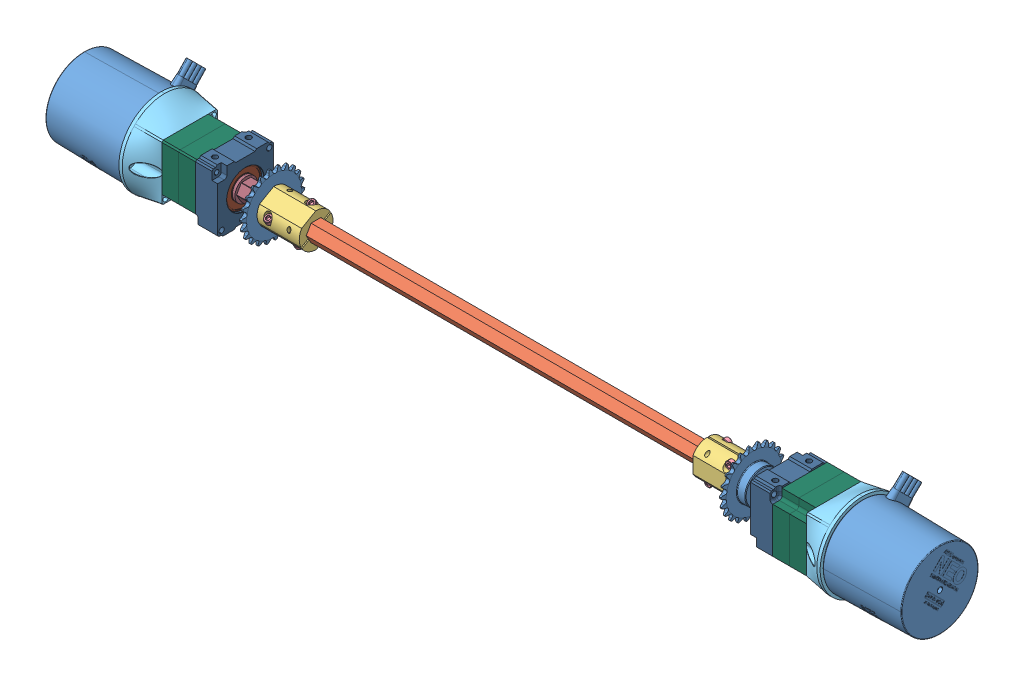
SolidWorks assembly elevator motors, configuration Default. Lengths in mm.
Overall size (645.18 70.15 70.15).
85 component instances, 19 part files, 27 mates.
Components (placement in the parent):
- 22t 25chain gear-1: 22t 25chain gear [Default] at (47.9906 -700.1428 1835.7253) x (-1 0 0) z (0 0.939892 -0.341472) size (9.18 48.36 48.44)
- 22t 25chain gear-2: 22t 25chain gear [Default] at (707.3859 453.67 -162.8689) x (1 0 0) z (0 0.174223 0.984706) size (9.18 48.36 48.44)
- 12in .5hex-1: 12in .5hex [Default] at (534.901 182.7836 1013.2629) x (0 0.972924 0.231127) z (-1 0 0) size (14.05 14.27 317.5)
- TTB-0055 - Half Inch Hex Coupler.stp-1: TTB-0055 - Half Inch Hex Coupler.stp [Default] at (230.101 182.8852 1013.3216) x (0 0.5 -0.866025) z (-1 0 0) size (26 22.23 31.75)
  - 6-32 Hex Coupler.stp-1: 6-32 Hex Coupler.stp [Default] at origin size (25.37 10.53 31.75)
  - 6-32 Hex Coupler.stp-2: 6-32 Hex Coupler.stp [Default] at (0 0 31.75) x (1 0 0) z (0 0 -1) size (25.37 10.53 31.75)
  - 91251A146_Black-Oxide Alloy Steel Socket Head Screw.stp-1: 91251A146_Black-Oxide Alloy Steel Socket Head Screw.stp [Default] at (9.5758 -1.5621 7.9375) x (0.375209 0 0.92694) z (0 -1 0) size (5.74 5.74 13.03)
  - 91251A146_Black-Oxide Alloy Steel Socket Head Screw.stp-2: 91251A146_Black-Oxide Alloy Steel Socket Head Screw.stp [Default] at (9.5758 1.5621 23.8125) x (-0.044233 0 -0.999021) z (0 1 0) size (5.74 5.74 13.03)
  - 91251A146_Black-Oxide Alloy Steel Socket Head Screw.stp-3: 91251A146_Black-Oxide Alloy Steel Socket Head Screw.stp [Default] at (-9.5758 -1.5621 23.8125) x (1 0 0) z (0 -1 0) size (5.74 5.74 13.03)
  - 91251A146_Black-Oxide Alloy Steel Socket Head Screw.stp-4: 91251A146_Black-Oxide Alloy Steel Socket Head Screw.stp [Default] at (-9.5758 1.5621 7.9375) x (1 0 0) z (0 1 0) size (5.74 5.74 13.03)
- TTB-0055 - Half Inch Hex Coupler.stp-2: TTB-0055 - Half Inch Hex Coupler.stp [Default] at (525.2756 182.8852 1013.3216) x (0 1 0) z (1 0 0) size (26 22.23 31.75)
  - 6-32 Hex Coupler.stp-1: 6-32 Hex Coupler.stp [Default] at origin size (25.37 10.53 31.75)
  - 6-32 Hex Coupler.stp-2: 6-32 Hex Coupler.stp [Default] at (0 0 31.75) x (1 0 0) z (0 0 -1) size (25.37 10.53 31.75)
  - 91251A146_Black-Oxide Alloy Steel Socket Head Screw.stp-1: 91251A146_Black-Oxide Alloy Steel Socket Head Screw.stp [Default] at (9.5758 -1.5621 7.9375) x (0.375209 0 0.92694) z (0 -1 0) size (5.74 5.74 13.03)
  - 91251A146_Black-Oxide Alloy Steel Socket Head Screw.stp-2: 91251A146_Black-Oxide Alloy Steel Socket Head Screw.stp [Default] at (9.5758 1.5621 23.8125) x (-0.044233 0 -0.999021) z (0 1 0) size (5.74 5.74 13.03)
  - 91251A146_Black-Oxide Alloy Steel Socket Head Screw.stp-3: 91251A146_Black-Oxide Alloy Steel Socket Head Screw.stp [Default] at (-9.5758 -1.5621 23.8125) x (1 0 0) z (0 -1 0) size (5.74 5.74 13.03)
  - 91251A146_Black-Oxide Alloy Steel Socket Head Screw.stp-4: 91251A146_Black-Oxide Alloy Steel Socket Head Screw.stp [Default] at (-9.5758 1.5621 7.9375) x (1 0 0) z (0 1 0) size (5.74 5.74 13.03)
- VersaPlanetary CIM Adapter (217-4018).step-1: VersaPlanetary CIM Adapter (217-4018).step [Default] at (630.4008 182.9868 1013.2629) x (0 0 1) z (0 -1 0) size (64.01 21.63 64.01)
- VersaPlanetary CIM Adapter (217-4018).step-2: VersaPlanetary CIM Adapter (217-4018).step [Default] at (124.9758 182.9868 1013.2629) x (0 0 1) z (0 1 0) size (64.01 21.63 64.01)
- Copy of Copy (2) of Assem5^elevator motors-1: Copy of Copy (2) of Assem5^elevator motors [Default] at (160.2008 205.2118 1013.2629) x (1 0 0) z (0 0 -1) size (98.55 51.52 52.65) (virtual)
  - 217-2820 Rev1_Public.step-1: 217-2820 Rev1_Public.step [Default] at (-4.6546 22.225 0) x (0 -0.456494 0.889726) z (-1 0 0) size (39.22 38.88 17.4)
    - 217-2625-100.step-1: 217-2625-100.step [Default] at origin size (39.22 38.88 12.7)
      - 217-2625-008 Rev1.step-1: 217-2625-008 Rev1.step [Default] at origin size (34.7 34.7 4.7)
      - 217-2625-010 Rev1.step-1: 217-2625-010 Rev1.step [Default] at (0 10.193 3.65) x (0.999813 0.019336 0) z (0 0 1) size (4 4 12)
      - 217-2625-010 Rev1.step-2: 217-2625-010 Rev1.step [Default] at (8.691 -5.3258 3.65) size (4 4 12)
      - 217-2625-010 Rev1.step-3: 217-2625-010 Rev1.step [Default] at (-8.691 -5.3258 3.65) size (4 4 12)
      - 217-2625-005 Rev1_Planet_Revolving_Follower01.step-1: 217-2625-005 Rev1_Planet_Revolving_Follower01.step [Default] at (8.691 -5.3258 6.35) x (0.932816 0.360354 0) z (0 0 1) size (16.89 16.89 8)
      - 217-2625-005 Rev1_Planet_Revolving_Follower01.step-2: 217-2625-005 Rev1_Planet_Revolving_Follower01.step [Default] at (-8.691 -5.3258 6.35) x (-0.932788 -0.360426 0) z (0 0 1) size (16.89 16.89 8)
      - 217-2625-005 Rev1_Planet_Revolving_Follower01.step-3: 217-2625-005 Rev1_Planet_Revolving_Follower01.step [Default] at (0 10.193 6.35) x (0.893583 0.448898 0) z (0 0 1) size (16.89 16.89 8)
    - 217-2625-007 Rev1_Public.step-1: 217-2625-007 Rev1_Public.step [Default] at (0 0 6.7) x (0.992772 0.120019 0) z (0 0 1) size (15.27 15.27 12.7)
  - 217-2820 Rev1_Public.step-2: 217-2820 Rev1_Public.step [Default] at (-17.15 22.225 0) x (0 0.184082 0.982911) z (-1 0 0) size (39.22 38.88 17.4)
    - 217-2625-100.step-1: 217-2625-100.step [Default] at origin size (39.22 38.88 12.7)
      - 217-2625-008 Rev1.step-1: 217-2625-008 Rev1.step [Default] at origin size (34.7 34.7 4.7)
      - 217-2625-010 Rev1.step-1: 217-2625-010 Rev1.step [Default] at (0 10.193 3.65) x (0.999813 0.019336 0) z (0 0 1) size (4 4 12)
      - 217-2625-010 Rev1.step-2: 217-2625-010 Rev1.step [Default] at (8.691 -5.3258 3.65) size (4 4 12)
      - 217-2625-010 Rev1.step-3: 217-2625-010 Rev1.step [Default] at (-8.691 -5.3258 3.65) size (4 4 12)
      - 217-2625-005 Rev1_Planet_Revolving_Follower01.step-1: 217-2625-005 Rev1_Planet_Revolving_Follower01.step [Default] at (8.691 -5.3258 6.35) x (0.932816 0.360354 0) z (0 0 1) size (16.89 16.89 8)
      - 217-2625-005 Rev1_Planet_Revolving_Follower01.step-2: 217-2625-005 Rev1_Planet_Revolving_Follower01.step [Default] at (-8.691 -5.3258 6.35) x (-0.932788 -0.360426 0) z (0 0 1) size (16.89 16.89 8)
      - 217-2625-005 Rev1_Planet_Revolving_Follower01.step-3: 217-2625-005 Rev1_Planet_Revolving_Follower01.step [Default] at (0 10.193 6.35) x (0.893583 0.448898 0) z (0 0 1) size (16.89 16.89 8)
    - 217-2625-007 Rev1_Public.step-1: 217-2625-007 Rev1_Public.step [Default] at (0 0 6.7) x (0.992772 0.120019 0) z (0 0 1) size (15.27 15.27 12.7)
  - 217-2625-026 Rev1.step-1: 217-2625-026 Rev1.step [Default] at (-6.5 22.225 0) x (0 -1 0) z (-1 0 0) size (44.45 42 18.12)
  - 217-2742-001 Rev4.step-1: 217-2742-001 Rev4.step [Default] at (0.2002 22.225 0) x (1 0 0) z (0 -0.092627 0.995701) size (7 28 28)
  - 217-2742-001 Rev4.step-2: 217-2742-001 Rev4.step [Default] at (8.2002 22.225 0) size (7 28 28)
  - 217-2625-017 Rev1_9714K61.step-1: 217-2625-017 Rev1_9714K61.step [Default] at (7.42 22.3002 -0.342) x (0 0.56703 0.823697) z (0 -0.823697 0.56703) size (28.51 4.98 27.43)
  - 217-2625-003 Rev1.step-1: 217-2625-003 Rev1.step [Default] at (7.4478 22.225 0) x (0 -1 0) z (1 0 0) size (17 17 64.11)
  - 217-2625-018 Rev1_98541A410.step-1: 217-2625-018 Rev1_98541A410.step [Default] at (-0.7046 22.225 0) x (1 0 0) z (0 -0.017452 0.999848) size (1 19.6 17.4)
  - 217-2816-001 Rev1.step-1: 217-2816-001 Rev1.step [Default] at (-6.35 22.225 0) x (0 -1 0) z (1 0 0) size (42 42 14.51)
  - 217-2816-001 Rev1.step-2: 217-2816-001 Rev1.step [Default] at (-19.05 22.225 0) x (0 -1 0) z (1 0 0) size (42 42 14.51)
  - 217-4649-001 Rev1.step-1: 217-4649-001 Rev1.step [Default] at (-32.746 22.225 0) x (0 -1 0) z (1 0 0) size (18 18 13)
  - 217-4649-007 Rev1_94105A824.step-1: 217-4649-007 Rev1_94105A824.step [Default] at (-38.221 22.225 -6.7835) x (-0.996104 -0.088191 0) z (0 0 -1) size (4.83 4.83 4.77)
  - 217-2625-011 Rev1.step-1: 217-2625-011 Rev1.step [Default] at (-37.4818 22.225 0) x (0 0 1) z (0 -1 0) size (8.01 7.5 7.94)
- Copy of Copy of Assem5^elevator motors-1: Copy of Copy of Assem5^elevator motors [Default] at (595.1758 205.2118 1013.2629) x (-1 0 0) z (0 0 1) size (98.55 51.52 52.65) (virtual)
  - 217-2820 Rev1_Public.step-1: 217-2820 Rev1_Public.step [Default] at (-4.6546 22.225 0) x (0 -0.456494 0.889726) z (-1 0 0) size (39.22 38.88 17.4)
    - 217-2625-100.step-1: 217-2625-100.step [Default] at origin size (39.22 38.88 12.7)
      - 217-2625-008 Rev1.step-1: 217-2625-008 Rev1.step [Default] at origin size (34.7 34.7 4.7)
      - 217-2625-010 Rev1.step-1: 217-2625-010 Rev1.step [Default] at (0 10.193 3.65) x (0.999813 0.019336 0) z (0 0 1) size (4 4 12)
      - 217-2625-010 Rev1.step-2: 217-2625-010 Rev1.step [Default] at (8.691 -5.3258 3.65) size (4 4 12)
      - 217-2625-010 Rev1.step-3: 217-2625-010 Rev1.step [Default] at (-8.691 -5.3258 3.65) size (4 4 12)
      - 217-2625-005 Rev1_Planet_Revolving_Follower01.step-1: 217-2625-005 Rev1_Planet_Revolving_Follower01.step [Default] at (8.691 -5.3258 6.35) x (0.932816 0.360354 0) z (0 0 1) size (16.89 16.89 8)
      - 217-2625-005 Rev1_Planet_Revolving_Follower01.step-2: 217-2625-005 Rev1_Planet_Revolving_Follower01.step [Default] at (-8.691 -5.3258 6.35) x (-0.932788 -0.360426 0) z (0 0 1) size (16.89 16.89 8)
      - 217-2625-005 Rev1_Planet_Revolving_Follower01.step-3: 217-2625-005 Rev1_Planet_Revolving_Follower01.step [Default] at (0 10.193 6.35) x (0.893583 0.448898 0) z (0 0 1) size (16.89 16.89 8)
    - 217-2625-007 Rev1_Public.step-1: 217-2625-007 Rev1_Public.step [Default] at (0 0 6.7) x (0.992772 0.120019 0) z (0 0 1) size (15.27 15.27 12.7)
  - 217-2820 Rev1_Public.step-2: 217-2820 Rev1_Public.step [Default] at (-17.15 22.225 0) x (0 0.184082 0.982911) z (-1 0 0) size (39.22 38.88 17.4)
    - 217-2625-100.step-1: 217-2625-100.step [Default] at origin size (39.22 38.88 12.7)
      - 217-2625-008 Rev1.step-1: 217-2625-008 Rev1.step [Default] at origin size (34.7 34.7 4.7)
      - 217-2625-010 Rev1.step-1: 217-2625-010 Rev1.step [Default] at (0 10.193 3.65) x (0.999813 0.019336 0) z (0 0 1) size (4 4 12)
      - 217-2625-010 Rev1.step-2: 217-2625-010 Rev1.step [Default] at (8.691 -5.3258 3.65) size (4 4 12)
      - 217-2625-010 Rev1.step-3: 217-2625-010 Rev1.step [Default] at (-8.691 -5.3258 3.65) size (4 4 12)
      - 217-2625-005 Rev1_Planet_Revolving_Follower01.step-1: 217-2625-005 Rev1_Planet_Revolving_Follower01.step [Default] at (8.691 -5.3258 6.35) x (0.932816 0.360354 0) z (0 0 1) size (16.89 16.89 8)
      - 217-2625-005 Rev1_Planet_Revolving_Follower01.step-2: 217-2625-005 Rev1_Planet_Revolving_Follower01.step [Default] at (-8.691 -5.3258 6.35) x (-0.932788 -0.360426 0) z (0 0 1) size (16.89 16.89 8)
      - 217-2625-005 Rev1_Planet_Revolving_Follower01.step-3: 217-2625-005 Rev1_Planet_Revolving_Follower01.step [Default] at (0 10.193 6.35) x (0.893583 0.448898 0) z (0 0 1) size (16.89 16.89 8)
    - 217-2625-007 Rev1_Public.step-1: 217-2625-007 Rev1_Public.step [Default] at (0 0 6.7) x (0.992772 0.120019 0) z (0 0 1) size (15.27 15.27 12.7)
  - 217-2625-026 Rev1.step-1: 217-2625-026 Rev1.step [Default] at (-6.5 22.225 0) x (0 -1 0) z (-1 0 0) size (44.45 42 18.12)
  - 217-2742-001 Rev4.step-1: 217-2742-001 Rev4.step [Default] at (0.2002 22.225 0) x (1 0 0) z (0 -0.092627 0.995701) size (7 28 28)
  - 217-2742-001 Rev4.step-2: 217-2742-001 Rev4.step [Default] at (8.2002 22.225 0) size (7 28 28)
  - 217-2625-017 Rev1_9714K61.step-1: 217-2625-017 Rev1_9714K61.step [Default] at (7.42 22.3002 -0.342) x (0 0.56703 0.823697) z (0 -0.823697 0.56703) size (28.51 4.98 27.43)
  - 217-2625-003 Rev1.step-1: 217-2625-003 Rev1.step [Default] at (7.4478 22.225 0) x (0 -1 0) z (1 0 0) size (17 17 64.11)
  - 217-2625-018 Rev1_98541A410.step-1: 217-2625-018 Rev1_98541A410.step [Default] at (-0.7046 22.225 0) x (1 0 0) z (0 -0.017452 0.999848) size (1 19.6 17.4)
  - 217-2816-001 Rev1.step-1: 217-2816-001 Rev1.step [Default] at (-6.35 22.225 0) x (0 -1 0) z (1 0 0) size (42 42 14.51)
  - 217-2816-001 Rev1.step-2: 217-2816-001 Rev1.step [Default] at (-19.05 22.225 0) x (0 -1 0) z (1 0 0) size (42 42 14.51)
  - 217-4649-001 Rev1.step-1: 217-4649-001 Rev1.step [Default] at (-32.746 22.225 0) x (0 -1 0) z (1 0 0) size (18 18 13)
  - 217-4649-007 Rev1_94105A824.step-1: 217-4649-007 Rev1_94105A824.step [Default] at (-38.221 22.225 -6.7835) x (-0.996104 -0.088191 0) z (0 0 -1) size (4.83 4.83 4.77)
  - 217-2625-011 Rev1.step-1: 217-2625-011 Rev1.step [Default] at (-37.4818 22.225 0) x (0 0 1) z (0 -1 0) size (8.01 7.5 7.94)
- REV-21-1650-V1.1.step-1: REV-21-1650-V1.1.step [Default] at (113.4508 182.9868 1013.2629) x (0 -1 0) z (1 0 0) size (68.13 68.01 93.35)
- REV-21-1650-V1.1.step-2: REV-21-1650-V1.1.step [Default] at (641.9258 182.9868 1013.2629) x (0 0 1) z (-1 0 0) size (68.13 68.01 93.35)
Mates (geometry in assembly coordinates):
- Coincident149: coincident anti-aligned: plane of Copy of Copy (2) of Assem5^Assem2_short elevator(1)-1/217-2625-003 Rev1.step-1 through (217.401 182.9868 1005.9306) normal (0 0.5 -0.866025); plane of 22t 25chain gear-1 through (189.1742 189.3495 1009.6041) normal (0 -0.5 0.866025)
- Coincident150: coincident anti-aligned: plane of Copy of Copy (2) of Assem5^Assem2_short elevator(1)-1/217-2625-003 Rev1.step-1 through (217.401 176.6368 1009.5967) normal (0 -0.5 -0.866025); plane of 22t 25chain gear-1 through (189.1742 182.9868 1005.9306) normal (0 0.5 0.866025)
- Coincident151: coincident anti-aligned: plane of TTB-0055 - Half Inch Hex Coupler.stp-1/6-32 Hex Coupler.stp-2 through (198.351 182.8852 1013.3216) normal (-1 0 0); plane of 22t 25chain gear-1 through (198.351 182.9868 1013.2776) normal (1 0 0)
- Coincident146: coincident anti-aligned: plane of Copy of Copy of Assem5^Assem2_short elevator(1)-1/217-2625-003 Rev1.step-1 through (537.9756 189.3368 1016.9291) normal (0 1 0); plane of 22t 25chain gear-2 through (566.2023 189.3368 1009.4941) normal (0 -1 0)
- Coincident147: coincident anti-aligned: plane of 12in .5hex-1 through (217.401 182.7836 1005.9306) normal (0 -0.5 -0.866025); plane of 22t 25chain gear-2 through (566.2023 176.6114 1009.4941) normal (0 0.5 0.866025)
- Coincident148: coincident anti-aligned: plane of TTB-0055 - Half Inch Hex Coupler.stp-2/6-32 Hex Coupler.stp-1 through (557.0256 182.8852 1013.3216) normal (1 0 0); plane of 22t 25chain gear-2 through (557.0256 182.9741 1013.1676) normal (-1 0 0)
- Coincident141: coincident anti-aligned: plane of TTB-0055 - Half Inch Hex Coupler.stp-2/6-32 Hex Coupler.stp-1 through (525.2756 182.8852 1005.8719) normal (0 0.5 0.866025); plane of 12in .5hex-1 through (217.401 182.7836 1005.9306) normal (0 -0.5 -0.866025)
- Coincident143: coincident anti-aligned: plane of TTB-0055 - Half Inch Hex Coupler.stp-2/6-32 Hex Coupler.stp-1 through (525.2756 176.4336 1009.5967) normal (0 1 0); plane of 12in .5hex-1 through (217.401 176.4336 1009.5967) normal (0 -1 0)
- Coincident145: coincident anti-aligned: plane of Copy of Copy (2) of Assem5^Assem2_short elevator(1)-1/217-2625-003 Rev1.step-1 through (217.401 176.6368 1009.5967) normal (1 0 0); plane of 12in .5hex-1 through (217.401 182.7836 1013.2629) normal (-1 0 0)
- Coincident137: coincident anti-aligned: plane of Copy of Copy (2) of Assem5^Assem2_short elevator(1)-1/217-2625-003 Rev1.step-1 through (217.401 189.3368 1009.5967) normal (0 1 0); plane of TTB-0055 - Half Inch Hex Coupler.stp-1/6-32 Hex Coupler.stp-1 through (230.101 189.3368 1009.5967) normal (0 -1 0)
- Coincident138: coincident anti-aligned: plane of Copy of Copy (2) of Assem5^Assem2_short elevator(1)-1/217-2625-003 Rev1.step-1 through (217.401 182.9868 1005.9306) normal (0 0.5 -0.866025); plane of TTB-0055 - Half Inch Hex Coupler.stp-1/6-32 Hex Coupler.stp-1 through (230.101 182.8852 1005.8719) normal (0 -0.5 0.866025)
- Distance23: distance = 12.7 mm: plane of Copy of Copy (2) of Assem5^Assem2_short elevator(1)-1/217-2625-003 Rev1.step-1 through (217.401 176.6368 1009.5967) normal (1 0 0); line of TTB-0055 - Half Inch Hex Coupler.stp-1/6-32 Hex Coupler.stp-1 through (230.101 189.3368 1017.0464) axis (0 -0.866025 0.5)
- Coincident135: coincident anti-aligned: plane of Copy of Copy of Assem5^Assem2_short elevator(1)-1/217-2625-003 Rev1.step-1 through (537.9756 189.3368 1009.5967) normal (0 0.5 -0.866025); plane of TTB-0055 - Half Inch Hex Coupler.stp-2/6-32 Hex Coupler.stp-1 through (525.2756 189.3368 1009.5967) normal (0 -0.5 0.866025)
- Coincident136: coincident anti-aligned: plane of Copy of Copy of Assem5^Assem2_short elevator(1)-1/217-2625-003 Rev1.step-1 through (537.9756 189.3368 1016.9291) normal (0 1 0); plane of TTB-0055 - Half Inch Hex Coupler.stp-2/6-32 Hex Coupler.stp-1 through (525.2756 189.3368 1017.0464) normal (0 -1 0)
- Distance24: distance = 12.7 mm aligned: plane of Copy of Copy of Assem5^Assem2_short elevator(1)-1/217-2625-003 Rev1.step-1 through (537.9756 176.6368 1016.9291) normal (-1 0 0); plane of TTB-0055 - Half Inch Hex Coupler.stp-2/6-32 Hex Coupler.stp-2 through (525.2756 182.8852 1013.3216) normal (-1 0 0)
- Concentric11: concentric anti-aligned: circle of Copy of Copy of Assem5^Assem2_short elevator(1)-1/217-2816-001 Rev1.step-2; circle of VersaPlanetary CIM Adapter (217-4018).step-1
- Coincident128: coincident anti-aligned: plane of Copy of Copy of Assem5^Assem2_short elevator(1)-1/217-2816-001 Rev1.step-2 through (620.5758 203.9868 992.2629) normal (1 0 0); plane of VersaPlanetary CIM Adapter (217-4018).step-1 through (620.5758 182.9868 1013.2629) normal (-1 0 0)
- Coincident129: coincident aligned: line of Copy of Copy of Assem5^Assem2_short elevator(1)-1/217-2816-001 Rev1.step-2 through (620.5758 203.9868 1027.2629) axis (0 0 -1); line of VersaPlanetary CIM Adapter (217-4018).step-1 through (620.5758 203.9868 1033.2629) axis (0 0 -1)
- Concentric12: concentric aligned: circle of REV-21-1650-V1.1.step-2; circle of VersaPlanetary CIM Adapter (217-4018).step-1
- Concentric13: concentric aligned: cylinder of REV-21-1650-V1.1.step-2 through (641.9258 182.9868 987.8629) axis (-1 0 0) radius 2.0193; circle of VersaPlanetary CIM Adapter (217-4018).step-1
- Coincident131: coincident anti-aligned: plane of REV-21-1650-V1.1.step-2 through (641.9258 182.9868 1013.2629) normal (-1 0 0); plane of VersaPlanetary CIM Adapter (217-4018).step-1 through (641.9258 182.9868 1013.2629) normal (1 0 0)
- Concentric14: concentric anti-aligned: circle of Copy of Copy (2) of Assem5^Assem2_short elevator(1)-1/217-2816-001 Rev1.step-2; circle of VersaPlanetary CIM Adapter (217-4018).step-2
- Perpendicular3: perpendicular: line of Copy of Copy (2) of Assem5^Assem2_short elevator(1)-1/217-2816-001 Rev1.step-2 through (134.8008 203.9868 999.2629) axis (0 0 1); line of VersaPlanetary CIM Adapter (217-4018).step-2 through (134.8008 162.9868 992.2629) axis (0 1 0)
- Coincident133: coincident anti-aligned: plane of Copy of Copy (2) of Assem5^Assem2_short elevator(1)-1/217-2816-001 Rev1.step-2 through (134.8008 203.9868 1034.2629) normal (-1 0 0); plane of VersaPlanetary CIM Adapter (217-4018).step-2 through (134.8008 182.9868 1013.2629) normal (1 0 0)
- Concentric15: concentric aligned: circle of REV-21-1650-V1.1.step-1; circle of VersaPlanetary CIM Adapter (217-4018).step-2
- Concentric16: concentric aligned: cylinder of REV-21-1650-V1.1.step-1 through (113.4508 182.9868 987.8629) axis (1 0 0) radius 2.0193; circle of VersaPlanetary CIM Adapter (217-4018).step-2
- Coincident134: coincident anti-aligned: plane of REV-21-1650-V1.1.step-1 through (113.4508 182.9868 1013.2629) normal (1 0 0); plane of VersaPlanetary CIM Adapter (217-4018).step-2 through (113.4508 182.9868 1013.2629) normal (-1 0 0)
